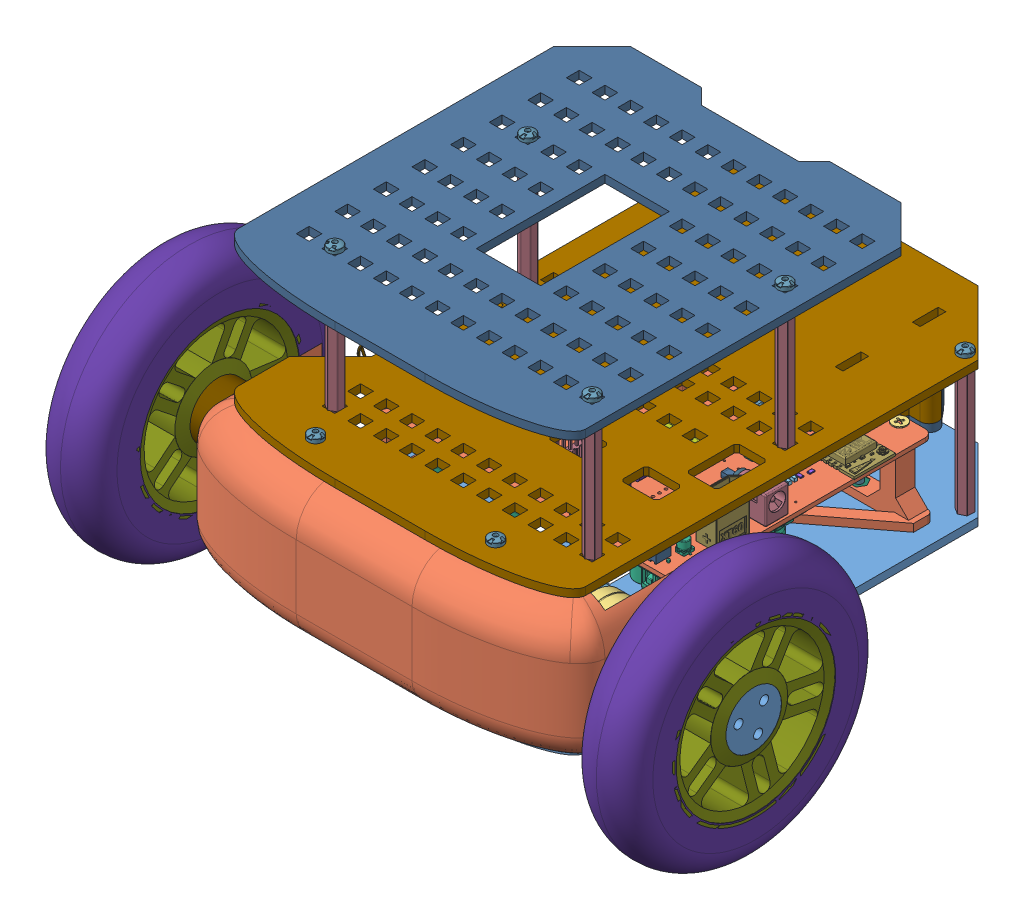
SolidWorks assembly assembly_base, configuration Default. Lengths in mm. (continued)
Components (placement in the parent): (continued)
- assembly_pcb_support-1: assembly_pcb_support [Default] at (108.2926 25.3704 228.3275) x (-1 0 0) z (0 0 -1) size (150.42 179.59 182.4) (continued)
  - noah_v02-1: noah_v02 [Default] at (-116.0171 92.6723 -13.0895) x (1 0 0) z (0 1 0) size (125.96 104.91 49.76) (continued)
    - noah_v02.step-1: noah_v02.step [Default] at origin size (125.96 104.91 49.76) (continued)
      - C_0603_1608Metric.step-4: C_0603_1608Metric.step [Default] at (156.1 -103.5 1.65) x (0.707107 -0.707107 0) z (0 0 1) size (1.6 0.8 0.8) (continued)
        - SOLID-31.step-1: SOLID-31.step [Default] at origin size (1.6 0.8 0.8)
      - C_0805_2012Metric.step-8: C_0805_2012Metric.step [Default] at (150.6 -113.5 1.65) x (-0.707107 -0.707107 0) z (0 0 1) size (2 1.25 1.25)
        - SOLID-1.step-1: SOLID-1.step [Default] at origin size (2 1.25 1.25)
      - C_0805_2012Metric.step-9: C_0805_2012Metric.step [Default] at (147.7 -116.4 1.65) x (0.707107 0.707107 0) z (0 0 1) size (2 1.25 1.25)
        - SOLID-1.step-1: SOLID-1.step [Default] at origin size (2 1.25 1.25)
      - C_0805_2012Metric.step-10: C_0805_2012Metric.step [Default] at (156.6 -108.9 1.65) x (-0.707107 -0.707107 0) z (0 0 1) size (2 1.25 1.25)
        - SOLID-1.step-1: SOLID-1.step [Default] at origin size (2 1.25 1.25)
      - C_1206_3216Metric.step-6: C_1206_3216Metric.step [Default] at (146.9 -123.1 1.65) x (-0.707107 -0.707107 0) z (0 0 1) size (3.2 1.6 1.6)
        - SOLID-32.step-1: SOLID-32.step [Default] at origin size (3.2 1.6 1.6)
      - C_0805_2012Metric.step-11: C_0805_2012Metric.step [Default] at (166 -103.2 1.65) x (0.707107 0.707107 0) z (0 0 1) size (2 1.25 1.25)
        - SOLID-1.step-1: SOLID-1.step [Default] at origin size (2 1.25 1.25)
      - C_0805_2012Metric.step-12: C_0805_2012Metric.step [Default] at (148.9 -124.3 1.65) x (0.707107 0.707107 0) z (0 0 1) size (2 1.25 1.25)
        - SOLID-1.step-1: SOLID-1.step [Default] at origin size (2 1.25 1.25)
      - C_0805_2012Metric.step-13: C_0805_2012Metric.step [Default] at (159.2 -134.3 1.65) x (0.707107 0.707107 0) z (0 0 1) size (2 1.25 1.25)
        - SOLID-1.step-1: SOLID-1.step [Default] at origin size (2 1.25 1.25)
      - C_0805_2012Metric.step-14: C_0805_2012Metric.step [Default] at (174.8 -116.6 1.65) x (-0.707107 -0.707107 0) z (0 0 1) size (2 1.25 1.25)
        - SOLID-1.step-1: SOLID-1.step [Default] at origin size (2 1.25 1.25)
      - CP_Elec_4x4.5.step-6: CP_Elec_4x4.5.step [Default] at (117.6 -66.1 1.65) x (-1 0 0) z (0 0 1) size (5.74 5.46 4.5)
        - SOLID-2.step-1: SOLID-2.step [Default] at origin size (5.74 5.46 4.5)
      - COMPOUND-33.step-1: COMPOUND-33.step [Default] at origin size (120 100 1.6)
  - countersunk flat head cross recess screw_din-1: countersunk flat head cross recess screw_din [DIN EN ISO 7046-1 - M3 x 10 - Z - 10C] at (90.2329 77.6723 137.4043) x (0 0 -1) z (-0.228588 0.973523 0) size (10 5.5 5.5)
  - countersunk flat head cross recess screw_din-2: countersunk flat head cross recess screw_din [DIN EN ISO 7046-1 - M3 x 10 - Z - 10C] at (90.9829 94.7761 133.9105) x (0 -1 0) z (0.969701 0 -0.244294) size (10 5.5 5.5)
  - countersunk flat head cross recess screw_din-4: countersunk flat head cross recess screw_din [DIN EN ISO 7046-1 - M3 x 10 - Z - 10C] at (90.2329 64.7046 111.9105) x (0 1 0) z (-0.097864 0 0.9952) size (10 5.5 5.5)
  - countersunk flat head cross recess screw_din-5: countersunk flat head cross recess screw_din [DIN EN ISO 7046-1 - M3 x 10 - Z - 10C] at (-16.0171 94.8904 133.9105) x (0 -1 0) z (-0.403912 0 0.914798) size (10 5.5 5.5)
  - countersunk flat head cross recess screw_din-6: countersunk flat head cross recess screw_din [DIN EN ISO 7046-1 - M3 x 10 - Z - 10C] at (90.9829 94.7842 39.9105) x (0 -1 0) z (-0.785339 0 -0.619066) size (10 5.5 5.5)
  - hex thin nut gradeb_din-1: hex thin nut gradeb_din [Hexagon Nut ISO 4036 - M3 - C] at (90.2329 67.4723 61.9105) x (0.5 0 -0.866025) z (0 1 0) size (5.5 6.35 1.8)
  - hex thin nut gradeb_din-2: hex thin nut gradeb_din [Hexagon Nut ISO 4036 - M3 - C] at (90.2329 65.6723 96.9105) x (0.5 0 -0.866025) z (0 -1 0) size (5.5 6.35 1.8)
  - hex thin nut gradeb_din-3: hex thin nut gradeb_din [Hexagon Nut ISO 4036 - M3 - C] at (68.9829 67.4723 133.1605) x (0.866025 0 -0.5) z (0 1 0) size (5.5 6.35 1.8)
  - hex thin nut gradeb_din-4: hex thin nut gradeb_din [Hexagon Nut ISO 4036 - M3 - C] at (-1.0171 65.6723 133.1605) x (0.866025 0 -0.5) z (0 -1 0) size (5.5 6.35 1.8)
  - assembly_button-1: assembly_button [Default] at (70.221 64.9929 125.1566) x (0 0 -1) z (1 0 0) size (25 20 8.52)
    - power_button_noah-1: power_button_noah [Default] at (5.7461 12.6794 16.2619) size (25 20 7.5)
    - LED 3mm Red 3mm Leads-1: LED 3mm Red 3mm Leads [Default] at (16.5561 8.6794 20.0119) x (0 1 0) z (-1 0 0) size (3.45 3.85 8.38)
      - LED 3mm Red 3mm Leads.step-1: LED 3mm Red 3mm Leads.step [Default] at origin size (3.45 3.85 8.38)
        - LEDBody.step-1: LEDBody.step [Default] at (0 0 0.01) size (3.45 3.85 5.38)
        - Lead1Body.step-1: Lead1Body.step [Default] at (0 0 0.01) size (0.5 0.5 3)
        - Lead2Body.step-1: Lead2Body.step [Default] at (0 0 0.01) size (0.5 0.5 3)
    - Tactile_Switch_SMD-1: Tactile_Switch_SMD [Default] at (5.7761 17.2044 15.4619) size (8 3.5 4.3)
    - LED 3mm Red 3mm Leads-2: LED 3mm Red 3mm Leads [Default] at (16.5561 16.6794 20.0119) x (0 1 0) z (-1 0 0) size (3.45 3.85 8.38)
      - LED 3mm Red 3mm Leads.step-1: LED 3mm Red 3mm Leads.step [Default] at origin size (3.45 3.85 8.38)
        - LEDBody.step-1: LEDBody.step [Default] at (0 0 0.01) size (3.45 3.85 5.38)
        - Lead1Body.step-1: Lead1Body.step [Default] at (0 0 0.01) size (0.5 0.5 3)
        - Lead2Body.step-1: Lead2Body.step [Default] at (0 0 0.01) size (0.5 0.5 3)
    - hex thin nut gradeb_din-1: hex thin nut gradeb_din [Hexagon Nut ISO 4036 - M3 - C] at (5.7461 5.9794 20.0119) x (1 0 0) z (0 1 0) size (5.5 6.35 1.8)
    - hex thin nut gradeb_din-2: hex thin nut gradeb_din [Hexagon Nut ISO 4036 - M3 - C] at (-0.9539 12.6794 20.0119) x (0 0.5 -0.866025) z (1 0 0) size (5.5 6.35 1.8)
- pan head cross recess screw_din-11: pan head cross recess screw_din [DIN EN ISO 7045 - M3 x 10 - Z - 10N] at (18.0597 84.6427 131.4169) x (0 1 0) z (0.173681 0 -0.984802) size (12.31 5.6 5.6)
- pan head cross recess screw_din-12: pan head cross recess screw_din [DIN EN ISO 7045 - M3 x 10 - Z - 10N] at (39.3097 84.6427 95.1669) x (0 1 0) z (0.999394 0 -0.034811) size (12.31 5.6 5.6)
- pan head cross recess screw_din-13: pan head cross recess screw_din [DIN EN ISO 7045 - M3 x 10 - Z - 10N] at (18.0597 84.6427 166.4169) x (0 1 0) z (0.995776 0 -0.091816) size (12.31 5.6 5.6)
- pan head cross recess screw_din-14: pan head cross recess screw_din [DIN EN ISO 7045 - M3 x 10 - Z - 10N] at (109.3097 84.6427 95.1669) x (0 1 0) z (-0.546944 0 0.837169) size (12.31 5.6 5.6)
- top_noah-1: top_noah [Predeterminado] at (74.3097 140.0427 151.4169) size (135.31 3.5 190.25)
- pan head cross recess screw_din-15: pan head cross recess screw_din [DIN EN ISO 7045 - M3 x 10 - Z - 10N] at (27.795 145.4427 68.4169) x (0 -1 0) z (0 0 1) size (12.31 5.6 5.6)
- pan head cross recess screw_din-16: pan head cross recess screw_din [DIN EN ISO 7045 - M3 x 10 - Z - 10N] at (136.8097 145.4427 81.4169) x (0 -1 0) z (0 0 1) size (12.31 5.6 5.6)
- pan head cross recess screw_din-17: pan head cross recess screw_din [DIN EN ISO 7045 - M3 x 10 - Z - 10N] at (39.3097 145.4427 236.4169) x (0 -1 0) z (0 0 1) size (12.31 5.6 5.6)
- pan head cross recess screw_din-18: pan head cross recess screw_din [DIN EN ISO 7045 - M3 x 10 - Z - 10N] at (109.3097 145.4427 236.4169) x (0 -1 0) z (0 0 1) size (12.31 5.6 5.6)
- Spacer50mm-4: Spacer50mm [Varsayılan] at (32.3097 193.0427 221.9169) x (-0.866025 0 -0.5) z (-0.5 0 0.866025) size (5.71 56.2 5)
- Spacer50mm-5: Spacer50mm [Varsayılan] at (132.3097 193.0427 221.9169) x (-0.866025 0 -0.5) z (-0.5 0 0.866025) size (5.71 56.2 5)
- Spacer50mm-6: Spacer50mm [Varsayılan] at (32.3097 193.0427 146.9169) x (-0.866025 0 -0.5) z (-0.5 0 0.866025) size (5.71 56.2 5)
- Spacer50mm-7: Spacer50mm [Varsayılan] at (132.3097 193.0427 146.9169) x (-0.866025 0 -0.5) z (-0.5 0 0.866025) size (5.71 56.2 5)
- shelf_noah-1: shelf_noah [Default] at (74.3097 193.0427 171.4169) size (135.31 3.5 150.25)
- pan head cross recess screw_din-19: pan head cross recess screw_din [DIN EN ISO 7045 - M3 x 10 - Z - 10N] at (32.3097 198.4427 146.9169) x (0 -1 0) z (0 0 1) size (12.31 5.6 5.6)
- pan head cross recess screw_din-20: pan head cross recess screw_din [DIN EN ISO 7045 - M3 x 10 - Z - 10N] at (32.3097 198.4427 221.9169) x (0 -1 0) z (-0.924225 0 0.381849) size (12.31 5.6 5.6)
- pan head cross recess screw_din-21: pan head cross recess screw_din [DIN EN ISO 7045 - M3 x 10 - Z - 10N] at (132.3097 198.4427 221.9169) x (0 -1 0) z (0 0 1) size (12.31 5.6 5.6)
- pan head cross recess screw_din-22: pan head cross recess screw_din [DIN EN ISO 7045 - M3 x 10 - Z - 10N] at (132.3097 198.4427 146.9169) x (0 -1 0) z (0 0 1) size (12.31 5.6 5.6)
- hex thin nut gradeb_din-3: hex thin nut gradeb_din [Hexagon Nut ISO 4036 - M3 - C] at (32.3097 138.2427 146.9169) x (1 0 0) z (0 -1 0) size (5.5 6.35 1.8)
- hex thin nut gradeb_din-4: hex thin nut gradeb_din [Hexagon Nut ISO 4036 - M3 - C] at (132.3097 138.2427 146.9169) x (0.82484 0 0.565366) z (0 -1 0) size (5.5 6.35 1.8)
- hex thin nut gradeb_din-5: hex thin nut gradeb_din [Hexagon Nut ISO 4036 - M3 - C] at (132.3097 138.2427 221.9169) x (1 0 0) z (0 -1 0) size (5.5 6.35 1.8)
- hex thin nut gradeb_din-6: hex thin nut gradeb_din [Hexagon Nut ISO 4036 - M3 - C] at (32.3097 138.2427 221.9169) x (1 0 0) z (0 -1 0) size (5.5 6.35 1.8)
Mates (geometry in assembly coordinates):
- Coincident1: coincident anti-aligned: plane of base_noah-1 through (74.3097 90.0427 151.4169) normal (0 1 0); plane of assembly_front-1/front_noah-1 through (74.3097 90.0427 226.4169) normal (0 -1 0)
- Concentric1: concentric anti-aligned: cylinder of base_noah-1 through (24.3097 87.0427 236.4169) axis (0 1 0) radius 1.75; cylinder of assembly_front-1/front_noah-1 through (24.3097 100.0427 236.4169) axis (0 -1 0) radius 1.5
- Concentric2: concentric anti-aligned: cylinder of base_noah-1 through (124.3097 87.0427 236.4169) axis (0 1 0) radius 1.75; cylinder of assembly_front-1/front_noah-1 through (124.3097 100.0427 236.4169) axis (0 -1 0) radius 1.5
- Coincident2: coincident anti-aligned: plane of base_noah-1 through (74.3097 90.0427 151.4169) normal (0 1 0); plane of CasterJoint-1/C001-1 through (47.3097 90.0427 59.9169) normal (0 -1 0)
- Concentric3: concentric aligned: cylinder of base_noah-1 through (101.3097 86.7927 59.9169) axis (0 1 0) radius 1.75; cylinder of CasterJoint-1/C000-1 through (101.3097 90.0427 59.9169) axis (0 1 0) radius 1.5
- Concentric4: concentric aligned: cylinder of base_noah-1 through (47.3097 86.7927 59.9169) axis (0 1 0) radius 1.75; cylinder of CasterJoint-1/C000-1 through (47.3097 90.0427 59.9169) axis (0 1 0) radius 1.5
- Concentric5: concentric aligned: cylinder of base_noah-1 through (27.8097 86.7927 68.4169) axis (0 1 0) radius 1.75; cylinder of Spacer50mm-3 through (27.8097 88.8427 68.4169) axis (0 1 0) radius 1.3375
- Coincident3: coincident anti-aligned: plane of base_noah-1 through (74.3097 90.0427 151.4169) normal (0 1 0); plane of Spacer50mm-3 through (27.8097 90.0427 68.4169) normal (0 -1 0)
- Concentric6: concentric aligned: cylinder of base_noah-1 through (136.8097 86.7927 81.4169) axis (0 1 0) radius 1.75; cylinder of Spacer50mm-1 through (136.8097 88.8427 81.4169) axis (0 1 0) radius 1.3375
- Coincident4: coincident anti-aligned: plane of base_noah-1 through (74.3097 90.0427 151.4169) normal (0 1 0); plane of Spacer50mm-1 through (136.8097 90.0427 81.4169) normal (0 -1 0)
- Concentric9: concentric anti-aligned: cylinder of base_noah-1 through (46.8097 87.0427 201.4169) axis (0 1 0) radius 1.75; cylinder of pan head cross recess screw_din-5 through (46.8097 59.2427 201.4169) axis (0 -1 0) radius 1.5
- Coincident5: coincident anti-aligned: plane of base_noah-1 through (74.3097 87.0427 151.4169) normal (0 -1 0); plane of pan head cross recess screw_din-5 through (45.3097 87.0427 201.4169) normal (0 1 0)
- Concentric13: concentric anti-aligned: cylinder of base_noah-1 through (24.3097 87.0427 236.4169) axis (0 1 0) radius 1.75; cylinder of pan head cross recess screw_din-2 through (24.3097 59.2427 236.4169) axis (0 -1 0) radius 1.5
- Coincident6: coincident anti-aligned: plane of base_noah-1 through (74.3097 87.0427 151.4169) normal (0 -1 0); plane of pan head cross recess screw_din-2 through (23.5333 87.0427 237.7004) normal (0 1 0)
- Concentric14: concentric anti-aligned: cylinder of base_noah-1 through (101.8097 87.0427 201.4169) axis (0 1 0) radius 1.75; cylinder of pan head cross recess screw_din-4 through (101.8097 59.2427 201.4169) axis (0 -1 0) radius 1.5
- Concentric15: concentric anti-aligned: cylinder of base_noah-1 through (124.3097 87.0427 236.4169) axis (0 1 0) radius 1.75; cylinder of pan head cross recess screw_din-1 through (124.3097 59.2427 236.4169) axis (0 -1 0) radius 1.5
- Coincident7: coincident anti-aligned: plane of base_noah-1 through (74.3097 87.0427 151.4169) normal (0 -1 0); plane of pan head cross recess screw_din-4 through (100.3097 87.0427 201.4169) normal (0 1 0)
- Concentric16: concentric anti-aligned: cylinder of base_noah-1 through (101.3097 86.7927 59.9169) axis (0 1 0) radius 1.75; cylinder of pan head cross recess screw_din-3 through (101.3097 59.2427 59.9169) axis (0 -1 0) radius 1.5
- Coincident8: coincident anti-aligned: plane of base_noah-1 through (74.3097 87.0427 151.4169) normal (0 -1 0); plane of pan head cross recess screw_din-3 through (99.8097 87.0427 59.9169) normal (0 1 0)
- Coincident9: coincident anti-aligned: plane of base_noah-1 through (74.3097 87.0427 151.4169) normal (0 -1 0); plane of pan head cross recess screw_din-1 through (122.8097 87.0427 236.4169) normal (0 1 0)
- Concentric17: concentric anti-aligned: cylinder of base_noah-1 through (47.3097 86.7927 59.9169) axis (0 1 0) radius 1.75; cylinder of pan head cross recess screw_din-6 through (47.3097 59.2427 59.9169) axis (0 -1 0) radius 1.5
- Coincident10: coincident anti-aligned: plane of base_noah-1 through (74.3097 87.0427 151.4169) normal (0 -1 0); plane of pan head cross recess screw_din-6 through (45.8192 87.0427 60.0856) normal (0 1 0)
- Coincident11: coincident anti-aligned: plane of base_noah-1 through (74.3097 87.0427 151.4169) normal (0 -1 0); plane of hex thin nut gradeb_din-2 through (136.8097 87.0427 84.5924) normal (0 1 0)
- Concentric19: concentric aligned: circle of base_noah-1; circle of hex thin nut gradeb_din-2
- Coincident12: coincident anti-aligned: plane of base_noah-1 through (74.3097 87.0427 151.4169) normal (0 -1 0); plane of hex thin nut gradeb_din-1 through (27.8097 87.0427 71.5924) normal (0 1 0)
- Concentric20: concentric aligned: circle of base_noah-1; circle of hex thin nut gradeb_din-1
- Concentric22: concentric anti-aligned: cylinder of assembly_front-1/JA25-371-12V-1/Axis-1 through (160.8097 113.4427 216.4169) axis (-1 0 0) radius 2; cylinder of TuxsWheel100mm-1/Adapter1-1 through (173.8097 113.4427 216.4169) axis (1 0 0) radius 2.1
- Distance1: distance = 2 mm anti-aligned: plane of assembly_front-1/front_noah-1 through (151.8097 140.0427 196.4169) normal (1 0 0); plane of TuxsWheel100mm-1/Adapter1-1 through (153.8097 113.4427 216.4169) normal (-1 0 0)
- Concentric23: concentric anti-aligned: cylinder of assembly_front-1/JA25-371-12V-2/Axis-1 through (-12.1903 113.4427 216.4169) axis (1 0 0) radius 2; cylinder of TuxsWheel100mm-2/Adapter1-1 through (-25.1903 113.4427 216.4169) axis (-1 0 0) radius 2.1
- Distance2: distance = 2 mm anti-aligned: plane of TuxsWheel100mm-2/Adapter1-1 through (-5.1903 113.4427 216.4169) normal (1 0 0); plane of assembly_front-1/front_noah-1 through (-3.1903 140.0427 196.4169) normal (-1 0 0)
- Coincident15: coincident anti-aligned: plane of base_noah-1 through (74.3097 90.0427 151.4169) normal (0 1 0); plane of assembly_pcb_support-1/pcb_holder_noah-1 through (16.3097 90.0427 189.4169) normal (0 -1 0)
- Concentric29: concentric anti-aligned: cylinder of base_noah-1 through (18.0597 86.7927 166.4169) axis (0 1 0) radius 1.75; cylinder of assembly_pcb_support-1/pcb_holder_noah-1 through (18.0597 101.0427 166.4169) axis (0 -1 0) radius 1.5
- Concentric30: concentric anti-aligned: cylinder of base_noah-1 through (109.3097 86.7927 95.1669) axis (0 1 0) radius 1.75; cylinder of assembly_pcb_support-1/pcb_holder_noah-1 through (109.3097 101.0427 95.1669) axis (0 -1 0) radius 1.5
- Concentric32: concentric aligned: cylinder of assembly_pcb_support-1/hex thin nut gradeb_din-4 through (109.3097 92.8427 95.1669) axis (0 -1 0) radius 1.25; cylinder of pan head cross recess screw_din-14 through (109.3097 59.2427 95.1669) axis (0 -1 0) radius 1.5
- Coincident16: coincident anti-aligned: plane of base_noah-1 through (74.3097 87.0427 151.4169) normal (0 -1 0); plane of pan head cross recess screw_din-14 through (108.054 87.0427 94.3465) normal (0 1 0)
- Concentric33: concentric anti-aligned: cylinder of assembly_pcb_support-1/hex thin nut gradeb_din-3 through (39.3097 91.0427 95.1669) axis (0 1 0) radius 1.25; cylinder of pan head cross recess screw_din-12 through (39.3097 59.2427 95.1669) axis (0 -1 0) radius 1.5
- Coincident17: coincident anti-aligned: plane of base_noah-1 through (74.3097 87.0427 151.4169) normal (0 -1 0); plane of pan head cross recess screw_din-12 through (39.3619 87.0427 96.666) normal (0 1 0)
- Concentric34: concentric aligned: cylinder of assembly_pcb_support-1/hex thin nut gradeb_din-2 through (18.0597 92.8427 131.4169) axis (0 -1 0) radius 1.25; cylinder of pan head cross recess screw_din-11 through (18.0597 59.2427 131.4169) axis (0 -1 0) radius 1.5
- Coincident19: coincident anti-aligned: plane of base_noah-1 through (74.3097 87.0427 151.4169) normal (0 -1 0); plane of pan head cross recess screw_din-11 through (19.5369 87.0427 131.6775) normal (0 1 0)
- Concentric35: concentric anti-aligned: cylinder of base_noah-1 through (18.0597 86.7927 166.4169) axis (0 1 0) radius 1.75; cylinder of pan head cross recess screw_din-13 through (18.0597 59.2427 166.4169) axis (0 -1 0) radius 1.5
- Coincident20: coincident anti-aligned: plane of base_noah-1 through (74.3097 87.0427 151.4169) normal (0 -1 0); plane of pan head cross recess screw_din-13 through (18.1974 87.0427 167.9106) normal (0 1 0)
- Coincident21: coincident anti-aligned: plane of assembly_front-1/front_noah-1 through (74.3097 140.0427 226.4169) normal (0 1 0); plane of top_noah-1 through (74.3097 140.0427 151.4169) normal (0 -1 0)
- Concentric36: concentric aligned: cylinder of assembly_front-1/front_noah-1 through (39.3097 130.0427 236.4169) axis (0 1 0) radius 1.5; cylinder of top_noah-1 through (39.3097 133.0427 236.4169) axis (0 1 0) radius 1.75
- Concentric37: concentric aligned: cylinder of Spacer50mm-1 through (136.8097 134.0427 81.4169) axis (0 1 0) radius 1.365; cylinder of top_noah-1 through (136.8097 133.0427 81.4169) axis (0 1 0) radius 1.5
- Coincident22: coincident anti-aligned: plane of top_noah-1 through (74.3097 143.0427 151.4169) normal (0 1 0); plane of pan head cross recess screw_din-18 through (110.8097 143.0427 236.4169) normal (0 -1 0)
- Coincident23: coincident anti-aligned: plane of top_noah-1 through (74.3097 143.0427 151.4169) normal (0 1 0); plane of pan head cross recess screw_din-17 through (40.8097 143.0427 236.4169) normal (0 -1 0)
- Coincident24: coincident anti-aligned: plane of top_noah-1 through (74.3097 143.0427 151.4169) normal (0 1 0); plane of pan head cross recess screw_din-16 through (138.3097 143.0427 81.4169) normal (0 -1 0)
- Coincident25: coincident anti-aligned: plane of top_noah-1 through (74.3097 143.0427 151.4169) normal (0 1 0); plane of pan head cross recess screw_din-15 through (29.295 143.0427 68.4169) normal (0 -1 0)
- Concentric39: concentric aligned: cylinder of top_noah-1 through (136.8097 133.0427 81.4169) axis (0 1 0) radius 1.5; cylinder of pan head cross recess screw_din-16 through (136.8097 170.8427 81.4169) axis (0 1 0) radius 1.5
- Concentric40: concentric aligned: cylinder of top_noah-1 through (27.795 133.0427 68.4169) axis (0 1 0) radius 1.75; cylinder of pan head cross recess screw_din-15 through (27.795 170.8427 68.4169) axis (0 1 0) radius 1.5
- Concentric41: concentric aligned: cylinder of assembly_front-1/front_noah-1 through (39.3097 130.0427 236.4169) axis (0 1 0) radius 1.5; cylinder of pan head cross recess screw_din-17 through (39.3097 170.8427 236.4169) axis (0 1 0) radius 1.5
- Concentric42: concentric aligned: cylinder of assembly_front-1/front_noah-1 through (109.3097 130.0427 236.4169) axis (0 1 0) radius 1.5; cylinder of pan head cross recess screw_din-18 through (109.3097 170.8427 236.4169) axis (0 1 0) radius 1.5
- Coincident26: coincident anti-aligned: plane of top_noah-1 through (74.3097 143.0427 151.4169) normal (0 1 0); plane of Spacer50mm-7 through (132.3097 143.0427 146.9169) normal (0 -1 0)
- Coincident27: coincident anti-aligned: plane of top_noah-1 through (74.3097 143.0427 151.4169) normal (0 1 0); plane of Spacer50mm-6 through (32.3097 143.0427 146.9169) normal (0 -1 0)
- Coincident28: coincident anti-aligned: plane of top_noah-1 through (74.3097 143.0427 151.4169) normal (0 1 0); plane of Spacer50mm-5 through (132.3097 143.0427 221.9169) normal (0 -1 0)
- Coincident29: coincident anti-aligned: plane of top_noah-1 through (74.3097 143.0427 151.4169) normal (0 1 0); plane of Spacer50mm-4 through (32.3097 143.0427 221.9169) normal (0 -1 0)
- Coincident30: coincident: line of top_noah-1 through (134.8097 143.0427 149.4169) axis (0 0 -1); plane of Spacer50mm-7 through (134.8097 143.0427 145.4736) normal (1 0 0)
- Coincident35: coincident: line of top_noah-1 through (134.8097 143.0427 224.4169) axis (0 0 -1); plane of Spacer50mm-5 through (134.8097 143.0427 220.4736) normal (1 0 0)
- Coincident36: coincident: point of top_noah-1; unknown of Spacer50mm-5
- Coincident37: coincident: unknown of top_noah-1; unknown of Spacer50mm-7
- Coincident38: coincident: line of top_noah-1 through (34.8097 143.0427 224.4169) axis (0 0 -1); plane of Spacer50mm-4 through (34.8097 143.0427 220.4736) normal (1 0 0)
- Coincident39: coincident: unknown of top_noah-1; unknown of Spacer50mm-4
- Coincident40: coincident anti-aligned: line of top_noah-1 through (34.8097 143.0427 149.4169) axis (0 0 -1); line of Spacer50mm-6 through (34.8097 143.0427 145.589) axis (0 0 1)
- Coincident41: coincident: unknown of top_noah-1; unknown of Spacer50mm-6
- Coincident42: coincident anti-aligned: plane of Spacer50mm-5 through (132.3097 193.0427 221.9169) normal (0 1 0); plane of shelf_noah-1 through (74.3097 193.0427 171.4169) normal (0 -1 0)
- Coincident43: coincident aligned: plane of top_noah-1 through (141.8097 143.0427 56.4169) normal (1 0 0); plane of shelf_noah-1 through (141.8097 196.0427 96.4169) normal (1 0 0)
- Coincident44: coincident aligned: plane of top_noah-1 through (6.8097 143.0427 246.4169) normal (0 0 1); plane of shelf_noah-1 through (6.8097 196.0427 246.4169) normal (0 0 1)
- Coincident45: coincident anti-aligned: plane of shelf_noah-1 through (74.3097 196.0427 171.4169) normal (0 1 0); plane of pan head cross recess screw_din-22 through (133.8097 196.0427 146.9169) normal (0 -1 0)
- Coincident46: coincident anti-aligned: plane of shelf_noah-1 through (74.3097 196.0427 171.4169) normal (0 1 0); plane of pan head cross recess screw_din-21 through (133.8097 196.0427 221.9169) normal (0 -1 0)
- Coincident47: coincident anti-aligned: plane of shelf_noah-1 through (74.3097 196.0427 171.4169) normal (0 1 0); plane of pan head cross recess screw_din-19 through (33.8097 196.0427 146.9169) normal (0 -1 0)
- Coincident48: coincident anti-aligned: plane of shelf_noah-1 through (74.3097 196.0427 171.4169) normal (0 1 0); plane of pan head cross recess screw_din-20 through (32.8825 196.0427 223.3033) normal (0 -1 0)
- Concentric43: concentric aligned: circle of Spacer50mm-7; cylinder of pan head cross recess screw_din-22 through (132.3097 223.8427 146.9169) axis (0 1 0) radius 1.5
- Concentric44: concentric aligned: circle of Spacer50mm-6; cylinder of pan head cross recess screw_din-19 through (32.3097 223.8427 146.9169) axis (0 1 0) radius 1.5
- Concentric45: concentric aligned: circle of Spacer50mm-5; cylinder of pan head cross recess screw_din-21 through (132.3097 223.8427 221.9169) axis (0 1 0) radius 1.5
- Concentric46: concentric aligned: circle of Spacer50mm-4; cylinder of pan head cross recess screw_din-20 through (32.3097 223.8427 221.9169) axis (0 1 0) radius 1.5
- Concentric47: concentric anti-aligned: cylinder of Spacer50mm-7 through (132.3097 141.8427 146.9169) axis (0 1 0) radius 1.3375; cylinder of hex thin nut gradeb_din-4 through (132.3097 140.0427 146.9169) axis (0 -1 0) radius 1.25
- Coincident49: coincident anti-aligned: plane of top_noah-1 through (74.3097 140.0427 151.4169) normal (0 -1 0); plane of hex thin nut gradeb_din-4 through (130.5144 140.0427 149.5362) normal (0 1 0)
- Coincident50: coincident anti-aligned: plane of top_noah-1 through (74.3097 140.0427 151.4169) normal (0 -1 0); plane of hex thin nut gradeb_din-3 through (32.3097 140.0427 150.0924) normal (0 1 0)
- Coincident51: coincident anti-aligned: plane of top_noah-1 through (74.3097 140.0427 151.4169) normal (0 -1 0); plane of hex thin nut gradeb_din-5 through (132.3097 140.0427 225.0924) normal (0 1 0)
- Coincident52: coincident anti-aligned: plane of top_noah-1 through (74.3097 140.0427 151.4169) normal (0 -1 0); plane of hex thin nut gradeb_din-6 through (32.3097 140.0427 225.0924) normal (0 1 0)
- Concentric48: concentric anti-aligned: cylinder of Spacer50mm-6 through (32.3097 141.8427 146.9169) axis (0 1 0) radius 1.3375; cylinder of hex thin nut gradeb_din-3 through (32.3097 140.0427 146.9169) axis (0 -1 0) radius 1.25
- Concentric49: concentric anti-aligned: cylinder of Spacer50mm-5 through (132.3097 141.8427 221.9169) axis (0 1 0) radius 1.3375; cylinder of hex thin nut gradeb_din-5 through (132.3097 140.0427 221.9169) axis (0 -1 0) radius 1.25
- Concentric50: concentric anti-aligned: cylinder of Spacer50mm-4 through (32.3097 141.8427 221.9169) axis (0 1 0) radius 1.3375; cylinder of hex thin nut gradeb_din-6 through (32.3097 140.0427 221.9169) axis (0 -1 0) radius 1.25
